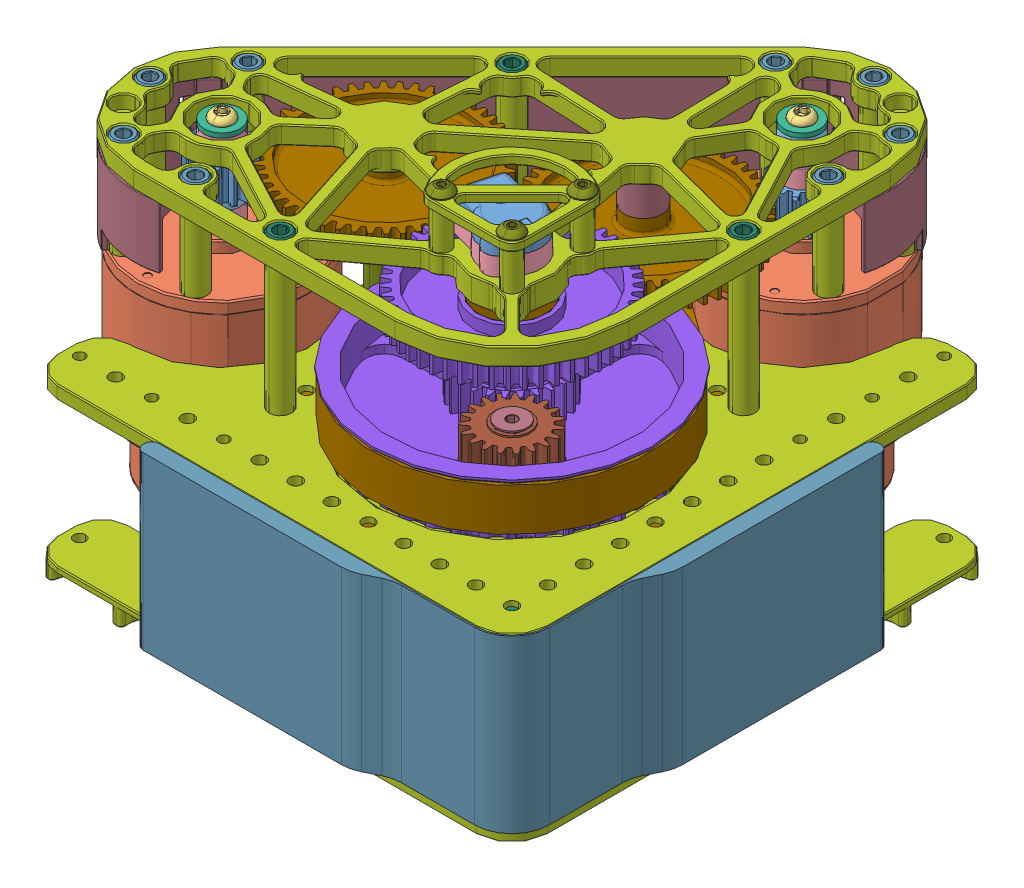
SolidWorks assembly SDS MK4i Swerve Module, Falcons, Independent, configuration Default. Lengths in mm.
Overall size (211.67 191.97 211.67).
99 component instances, 50 part files, 6 mates.
Components (placement in the parent):
- SDS MK4i Swerve Module, Falcons(2)^SDS MK4i Swerve Module, Falcons, Independent-2: SDS MK4i Swerve Module, Falcons(2)^SDS MK4i Swerve Module, Falcons, Independent [Default] at origin size (192.79 191.97 192.79) (virtual)
  - CANcoder Assembly^SDS MK4i Swerve Module, Falcons(2)_SDS MK4i Swerve Module, Falcons, Independent-1: CANcoder Assembly^SDS MK4i Swerve Module, Falcons(2)_SDS MK4i Swerve Module, Falcons, Independent [Default] at (-66.675 132.3975 -66.675) x (-0.260871 0 0.965374) z (0 1 0) size (21.75 26.91 13.52) (virtual)
    - CANcoder Top Housing^CANcoder Assembly_SDS MK4i Swerve Module, Falcons(2)_SDS MK4i Swerve Module, Falcons, Independent-1: CANcoder Top Housing^CANcoder Assembly_SDS MK4i Swerve Module, Falcons(2)_SDS MK4i Swerve Module, Falcons, Independent [Default] at origin size (21.53 26.79 8.94) (virtual)
    - CANcoder PCA^CANcoder Assembly_SDS MK4i Swerve Module, Falcons(2)_SDS MK4i Swerve Module, Falcons, Independent-1: CANcoder PCA^CANcoder Assembly_SDS MK4i Swerve Module, Falcons(2)_SDS MK4i Swerve Module, Falcons, Independent [Default] at (0 0 22.3055) size (15.93 23.27 3.19) (virtual)
    - CANcoder Screw^CANcoder Assembly_SDS MK4i Swerve Module, Falcons(2)_SDS MK4i Swerve Module, Falcons, Independent-1: CANcoder Screw^CANcoder Assembly_SDS MK4i Swerve Module, Falcons(2)_SDS MK4i Swerve Module, Falcons, Independent [Default] at origin size (4.24 4.24 12.65) (virtual)
    - CANcoder Bottom Housing^CANcoder Assembly_SDS MK4i Swerve Module, Falcons(2)_SDS MK4i Swerve Module, Falcons, Independent-1: CANcoder Bottom Housing^CANcoder Assembly_SDS MK4i Swerve Module, Falcons(2)_SDS MK4i Swerve Module, Falcons, Independent [Default] at origin size (21.75 26.91 6.35) (virtual)
  - MK4 Billet Wheel Assembly^SDS MK4i Swerve Module, Falcons(2)_SDS MK4i Swerve Module, Falcons, Independent-1: MK4 Billet Wheel Assembly^SDS MK4i Swerve Module, Falcons(2)_SDS MK4i Swerve Module, Falcons, Independent [Default] at (-66.675 50.7435 -66.675) x (0.707107 0 0.707107) z (0.41117 0.813559 -0.41117) size (42.28 100.13 100.13) (virtual)
    - Wheel, SDS, Nitrile Tread, 4in X 1.5in, Bearing Bore^MK4 Billet Wheel Assembly_SDS MK4i Swerve Module, Falcons(2)_SDS MK4i Swerve Module, Falcons, Independent-1: Wheel, SDS, Nitrile Tread, 4in X 1.5in, Bearing Bore^MK4 Billet Wheel Assembly_SDS MK4i Swerve Module, Falcons(2)_SDS MK4i Swerve Module, Falcons, Independent [Default] at origin size (42.28 88.9 88.9) (virtual)
    - Tread, Blue Nitrile 4in X 1.5in^MK4 Billet Wheel Assembly_SDS MK4i Swerve Module, Falcons(2)_SDS MK4i Swerve Module, Falcons, Independent-1: Tread, Blue Nitrile 4in X 1.5in^MK4 Billet Wheel Assembly_SDS MK4i Swerve Module, Falcons(2)_SDS MK4i Swerve Module, Falcons, Independent [Default] at origin size (38.1 100.13 100.13) (virtual)
    - Screw, 10-32 X .75, Button, 91255A269_91255A269^MK4 Billet Wheel Assembly_SDS MK4i Swerve Module, Falcons(2)_SDS MK4i Swerve Module, Falcons, Independent-1: Screw, 10-32 X .75, Button, 91255A269_91255A269^MK4 Billet Wheel Assembly_SDS MK4i Swerve Module, Falcons(2)_SDS MK4i Swerve Module, Falcons, Independent [Default] at (-4.826 0 20.6375) x (0 -0.847203 -0.531269) z (-1 0 0) size (9.17 9.17 21.62) (virtual)
    - Screw, 10-32 X .75, Button, 91255A269_91255A269^MK4 Billet Wheel Assembly_SDS MK4i Swerve Module, Falcons(2)_SDS MK4i Swerve Module, Falcons, Independent-2: Screw, 10-32 X .75, Button, 91255A269_91255A269^MK4 Billet Wheel Assembly_SDS MK4i Swerve Module, Falcons(2)_SDS MK4i Swerve Module, Falcons, Independent [Default] at (-4.826 -17.8726 10.3187) x (0 -0.99925 -0.038711) z (-1 0 0) size (9.17 9.17 21.62) (virtual)
    - Screw, 10-32 X .75, Button, 91255A269_91255A269^MK4 Billet Wheel Assembly_SDS MK4i Swerve Module, Falcons(2)_SDS MK4i Swerve Module, Falcons, Independent-3: Screw, 10-32 X .75, Button, 91255A269_91255A269^MK4 Billet Wheel Assembly_SDS MK4i Swerve Module, Falcons(2)_SDS MK4i Swerve Module, Falcons, Independent [Default] at (-4.826 -17.8726 -10.3187) x (0 -0.986188 -0.165633) z (-1 0 0) size (9.17 9.17 21.62) (virtual)
    - Screw, 10-32 X .75, Button, 91255A269_91255A269^MK4 Billet Wheel Assembly_SDS MK4i Swerve Module, Falcons(2)_SDS MK4i Swerve Module, Falcons, Independent-4: Screw, 10-32 X .75, Button, 91255A269_91255A269^MK4 Billet Wheel Assembly_SDS MK4i Swerve Module, Falcons(2)_SDS MK4i Swerve Module, Falcons, Independent [Default] at (-4.826 0 -20.6375) x (0 -0.966455 -0.256836) z (-1 0 0) size (9.17 9.17 21.62) (virtual)
    - Screw, 10-32 X .75, Button, 91255A269_91255A269^MK4 Billet Wheel Assembly_SDS MK4i Swerve Module, Falcons(2)_SDS MK4i Swerve Module, Falcons, Independent-5: Screw, 10-32 X .75, Button, 91255A269_91255A269^MK4 Billet Wheel Assembly_SDS MK4i Swerve Module, Falcons(2)_SDS MK4i Swerve Module, Falcons, Independent [Default] at (-4.826 17.8726 -10.3187) x (0 -0.95104 -0.309068) z (-1 0 0) size (9.17 9.17 21.62) (virtual)
    - Screw, 10-32 X .75, Button, 91255A269_91255A269^MK4 Billet Wheel Assembly_SDS MK4i Swerve Module, Falcons(2)_SDS MK4i Swerve Module, Falcons, Independent-6: Screw, 10-32 X .75, Button, 91255A269_91255A269^MK4 Billet Wheel Assembly_SDS MK4i Swerve Module, Falcons(2)_SDS MK4i Swerve Module, Falcons, Independent [Default] at (-4.826 17.8726 10.3187) x (0 -0.947988 -0.318305) z (-1 0 0) size (9.17 9.17 21.62) (virtual)
    - Screw, 10-32 X .5, Button, 97763A232_97763A232^MK4 Billet Wheel Assembly_SDS MK4i Swerve Module, Falcons(2)_SDS MK4i Swerve Module, Falcons, Independent-1: Screw, 10-32 X .5, Button, 97763A232_97763A232^MK4 Billet Wheel Assembly_SDS MK4i Swerve Module, Falcons(2)_SDS MK4i Swerve Module, Falcons, Independent [Default] at (11.1125 -40.6604 7.1695) x (-0.785325 0.107503 0.609678) z (0 -0.984808 0.173648) size (9.17 9.17 15.27) (virtual)
    - Screw, 10-32 X .5, Button, 97763A232_97763A232^MK4 Billet Wheel Assembly_SDS MK4i Swerve Module, Falcons(2)_SDS MK4i Swerve Module, Falcons, Independent-2: Screw, 10-32 X .5, Button, 97763A232_97763A232^MK4 Billet Wheel Assembly_SDS MK4i Swerve Module, Falcons(2)_SDS MK4i Swerve Module, Falcons, Independent [Default] at (-11.1125 -40.6604 7.1695) x (-0.636812 0.133886 0.759306) z (0 -0.984808 0.173648) size (9.17 9.17 15.27) (virtual)
    - Screw, 10-32 X .5, Button, 97763A232_97763A232^MK4 Billet Wheel Assembly_SDS MK4i Swerve Module, Falcons(2)_SDS MK4i Swerve Module, Falcons, Independent-3: Screw, 10-32 X .5, Button, 97763A232_97763A232^MK4 Billet Wheel Assembly_SDS MK4i Swerve Module, Falcons(2)_SDS MK4i Swerve Module, Falcons, Independent [Default] at (-11.1125 -40.6604 -7.1695) x (0.726076 -0.119403 0.677168) z (0 -0.984808 -0.173648) size (9.17 9.17 15.27) (virtual)
    - Screw, 10-32 X .5, Button, 97763A232_97763A232^MK4 Billet Wheel Assembly_SDS MK4i Swerve Module, Falcons(2)_SDS MK4i Swerve Module, Falcons, Independent-4: Screw, 10-32 X .5, Button, 97763A232_97763A232^MK4 Billet Wheel Assembly_SDS MK4i Swerve Module, Falcons(2)_SDS MK4i Swerve Module, Falcons, Independent [Default] at (11.1125 -40.6604 -7.1695) x (0.841108 -0.09392 0.53265) z (0 -0.984808 -0.173648) size (9.17 9.17 15.27) (virtual)
    - Screw, 10-32 X .5, Button, 97763A232_97763A232^MK4 Billet Wheel Assembly_SDS MK4i Swerve Module, Falcons(2)_SDS MK4i Swerve Module, Falcons, Independent-5: Screw, 10-32 X .5, Button, 97763A232_97763A232^MK4 Billet Wheel Assembly_SDS MK4i Swerve Module, Falcons(2)_SDS MK4i Swerve Module, Falcons, Independent [Default] at (-11.1125 20.6438 -35.7562) x (0.804058 -0.514897 -0.297276) z (0 0.5 -0.866025) size (9.17 9.17 15.27) (virtual)
    - Screw, 10-32 X .5, Button, 97763A232_97763A232^MK4 Billet Wheel Assembly_SDS MK4i Swerve Module, Falcons(2)_SDS MK4i Swerve Module, Falcons, Independent-6: Screw, 10-32 X .5, Button, 97763A232_97763A232^MK4 Billet Wheel Assembly_SDS MK4i Swerve Module, Falcons(2)_SDS MK4i Swerve Module, Falcons, Independent [Default] at (11.1125 20.6438 -35.7562) x (0.926716 -0.32542 -0.187881) z (0 0.5 -0.866025) size (9.17 9.17 15.27) (virtual)
    - Screw, 10-32 X .5, Button, 97763A232_97763A232^MK4 Billet Wheel Assembly_SDS MK4i Swerve Module, Falcons(2)_SDS MK4i Swerve Module, Falcons, Independent-7: Screw, 10-32 X .5, Button, 97763A232_97763A232^MK4 Billet Wheel Assembly_SDS MK4i Swerve Module, Falcons(2)_SDS MK4i Swerve Module, Falcons, Independent [Default] at (11.1125 20.6438 35.7562) x (0.200031 0.848523 -0.489895) z (0 0.5 0.866025) size (9.17 9.17 15.27) (virtual)
    - Screw, 10-32 X .5, Button, 97763A232_97763A232^MK4 Billet Wheel Assembly_SDS MK4i Swerve Module, Falcons(2)_SDS MK4i Swerve Module, Falcons, Independent-8: Screw, 10-32 X .5, Button, 97763A232_97763A232^MK4 Billet Wheel Assembly_SDS MK4i Swerve Module, Falcons(2)_SDS MK4i Swerve Module, Falcons, Independent [Default] at (-11.1125 20.6438 35.7562) x (0.515054 0.74232 -0.428579) z (0 0.5 0.866025) size (9.17 9.17 15.27) (virtual)
  - Screw, 10-32 X .25, Button, 91255A261_91255A261^SDS MK4i Swerve Module, Falcons(2)_SDS MK4i Swerve Module, Falcons, Independent-1: Screw, 10-32 X .25, Button, 91255A261_91255A261^SDS MK4i Swerve Module, Falcons(2)_SDS MK4i Swerve Module, Falcons, Independent [Default] at (-42.2285 89.5096 -114.6539) x (1 0 0) z (0 -1 0) size (9.17 9.17 8.92) (virtual)
  - Screw, 10-32 X .25, Button, 91255A261_91255A261^SDS MK4i Swerve Module, Falcons(2)_SDS MK4i Swerve Module, Falcons, Independent-2: Screw, 10-32 X .25, Button, 91255A261_91255A261^SDS MK4i Swerve Module, Falcons(2)_SDS MK4i Swerve Module, Falcons, Independent [Default] at (-104.7513 89.5096 -104.7513) x (0.982082 0 -0.188455) z (0 -1 0) size (9.17 9.17 8.92) (virtual)
  - Screw, 10-32 X .25, Button, 91255A261_91255A261^SDS MK4i Swerve Module, Falcons(2)_SDS MK4i Swerve Module, Falcons, Independent-3: Screw, 10-32 X .25, Button, 91255A261_91255A261^SDS MK4i Swerve Module, Falcons(2)_SDS MK4i Swerve Module, Falcons, Independent [Default] at (-114.6539 89.5096 -42.2285) x (0.918365 0 -0.395734) z (0 -1 0) size (9.17 9.17 8.92) (virtual)
  - Screw, 10-32 X .25, Button, 91255A261_91255A261^SDS MK4i Swerve Module, Falcons(2)_SDS MK4i Swerve Module, Falcons, Independent-4: Screw, 10-32 X .25, Button, 91255A261_91255A261^SDS MK4i Swerve Module, Falcons(2)_SDS MK4i Swerve Module, Falcons, Independent [Default] at (-63.5129 89.5096 -12.9199) x (0.8 0 -0.6) z (0 -1 0) size (9.17 9.17 8.92) (virtual)
  - Screw, 10-32 X .25, Button, 91255A261_91255A261^SDS MK4i Swerve Module, Falcons(2)_SDS MK4i Swerve Module, Falcons, Independent-5: Screw, 10-32 X .25, Button, 91255A261_91255A261^SDS MK4i Swerve Module, Falcons(2)_SDS MK4i Swerve Module, Falcons, Independent [Default] at (-12.9199 89.5096 -63.5129) x (0.63358 0 -0.773678) z (0 -1 0) size (9.17 9.17 8.92) (virtual)
  - Screw, Shoulder, .375 X 2.5, 5_16-18, 91259A634_91259A634^SDS MK4i Swerve Module, Falcons(2)_SDS MK4i Swerve Module, Falcons, Independent-1: Screw, Shoulder, .375 X 2.5, 5_16-18, 91259A634_91259A634^SDS MK4i Swerve Module, Falcons(2)_SDS MK4i Swerve Module, Falcons, Independent [Default] at (-93.8403 50.7435 -93.8403) x (-0.019195 -0.999631 0.019195) z (0.706846 -0.027146 -0.706846) size (14.29 82.55 14.29) (virtual)
  - Screw, .25-20 X 1 Socket, 91251A542_91251A542^SDS MK4i Swerve Module, Falcons(2)_SDS MK4i Swerve Module, Falcons, Independent-1: Screw, .25-20 X 1 Socket, 91251A542_91251A542^SDS MK4i Swerve Module, Falcons(2)_SDS MK4i Swerve Module, Falcons, Independent [Default] at (-102.596 101.6 -73.8592) x (0.964329 0 0.264706) z (0 1 0) size (9.53 9.53 31.75) (virtual)
  - Screw, .25-20 X 1 Socket, 91251A542_91251A542^SDS MK4i Swerve Module, Falcons(2)_SDS MK4i Swerve Module, Falcons, Independent-2: Screw, .25-20 X 1 Socket, 91251A542_91251A542^SDS MK4i Swerve Module, Falcons(2)_SDS MK4i Swerve Module, Falcons, Independent [Default] at (-73.8592 101.6 -102.596) x (0.982082 0 -0.188455) z (0 1 0) size (9.53 9.53 31.75) (virtual)
  - Screw, .25-20 X .625, 91251A539_91251A539^SDS MK4i Swerve Module, Falcons(2)_SDS MK4i Swerve Module, Falcons, Independent-1: Screw, .25-20 X .625, 91251A539_91251A539^SDS MK4i Swerve Module, Falcons(2)_SDS MK4i Swerve Module, Falcons, Independent [Default] at (-59.4908 83.2802 -30.754) x (1 0 0) z (0 -1 0) size (9.53 9.53 22.23) (virtual)
  - Screw, .25-20 X .625, 91251A539_91251A539^SDS MK4i Swerve Module, Falcons(2)_SDS MK4i Swerve Module, Falcons, Independent-2: Screw, .25-20 X .625, 91251A539_91251A539^SDS MK4i Swerve Module, Falcons(2)_SDS MK4i Swerve Module, Falcons, Independent [Default] at (-30.754 83.2802 -59.4908) x (0.982082 0 -0.188455) z (0 -1 0) size (9.53 9.53 22.23) (virtual)
  - Screw, .25-20 X .625, 91251A539_91251A539^SDS MK4i Swerve Module, Falcons(2)_SDS MK4i Swerve Module, Falcons, Independent-3: Screw, .25-20 X .625, 91251A539_91251A539^SDS MK4i Swerve Module, Falcons(2)_SDS MK4i Swerve Module, Falcons, Independent [Default] at (-66.675 126.2062 -66.675) x (0 0 1) z (0 1 0) size (9.53 9.53 22.23) (virtual)
  - Screw, 12-24 X .625, Flat, 91253A282_91253A282^SDS MK4i Swerve Module, Falcons(2)_SDS MK4i Swerve Module, Falcons, Independent-1: Screw, 12-24 X .625, Flat, 91253A282_91253A282^SDS MK4i Swerve Module, Falcons(2)_SDS MK4i Swerve Module, Falcons, Independent [Default] at (-46.8646 122.8979 -46.8646) x (-0.837169 0 -0.546944) z (0 1 0) size (10.72 10.72 15.88) (virtual)
  - Screw, 10-32 X 1.375, 90044A202_90044A202^SDS MK4i Swerve Module, Falcons(2)_SDS MK4i Swerve Module, Falcons, Independent-1: Screw, 10-32 X 1.375, 90044A202_90044A202^SDS MK4i Swerve Module, Falcons(2)_SDS MK4i Swerve Module, Falcons, Independent [Default] at (-34.518 138.8491 -146.05) x (-0.434408 0 0.900716) z (0 1 0) size (7.94 7.94 39.75) (virtual)
  - Screw, 10-32 X 1.375, 90044A202_90044A202^SDS MK4i Swerve Module, Falcons(2)_SDS MK4i Swerve Module, Falcons, Independent-2: Screw, 10-32 X 1.375, 90044A202_90044A202^SDS MK4i Swerve Module, Falcons(2)_SDS MK4i Swerve Module, Falcons, Independent [Default] at (-34.518 138.8491 -171.45) x (-0.25688 0 0.966443) z (0 1 0) size (7.94 7.94 39.75) (virtual)
  - Screw, 10-32 X 1.375, 90044A202_90044A202^SDS MK4i Swerve Module, Falcons(2)_SDS MK4i Swerve Module, Falcons, Independent-3: Screw, 10-32 X 1.375, 90044A202_90044A202^SDS MK4i Swerve Module, Falcons(2)_SDS MK4i Swerve Module, Falcons, Independent [Default] at (-56.515 138.8491 -184.15) x (-0.042501 0 0.999096) z (0 1 0) size (7.94 7.94 39.75) (virtual)
  - Screw, 10-32 X 1.375, 90044A202_90044A202^SDS MK4i Swerve Module, Falcons(2)_SDS MK4i Swerve Module, Falcons, Independent-4: Screw, 10-32 X 1.375, 90044A202_90044A202^SDS MK4i Swerve Module, Falcons(2)_SDS MK4i Swerve Module, Falcons, Independent [Default] at (-78.512 138.8491 -171.45) x (0.192903 0 0.981218) z (0 1 0) size (7.94 7.94 39.75) (virtual)
  - Screw, 10-32 X 1.375, 90044A202_90044A202^SDS MK4i Swerve Module, Falcons(2)_SDS MK4i Swerve Module, Falcons, Independent-5: Screw, 10-32 X 1.375, 90044A202_90044A202^SDS MK4i Swerve Module, Falcons(2)_SDS MK4i Swerve Module, Falcons, Independent [Default] at (-171.45 138.8491 -78.512) x (0.421632 0 0.906767) z (0 1 0) size (7.94 7.94 39.75) (virtual)
  - Screw, 10-32 X 1.375, 90044A202_90044A202^SDS MK4i Swerve Module, Falcons(2)_SDS MK4i Swerve Module, Falcons, Independent-6: Screw, 10-32 X 1.375, 90044A202_90044A202^SDS MK4i Swerve Module, Falcons(2)_SDS MK4i Swerve Module, Falcons, Independent [Default] at (-184.15 138.8491 -56.515) x (0.614515 0 0.788905) z (0 1 0) size (7.94 7.94 39.75) (virtual)
  - Screw, 10-32 X 1.375, 90044A202_90044A202^SDS MK4i Swerve Module, Falcons(2)_SDS MK4i Swerve Module, Falcons, Independent-7: Screw, 10-32 X 1.375, 90044A202_90044A202^SDS MK4i Swerve Module, Falcons(2)_SDS MK4i Swerve Module, Falcons, Independent [Default] at (-171.45 138.8491 -34.518) x (0.754605 0 0.656179) z (0 1 0) size (7.94 7.94 39.75) (virtual)
  - Screw, 10-32 X 1.375, 90044A202_90044A202^SDS MK4i Swerve Module, Falcons(2)_SDS MK4i Swerve Module, Falcons, Independent-8: Screw, 10-32 X 1.375, 90044A202_90044A202^SDS MK4i Swerve Module, Falcons(2)_SDS MK4i Swerve Module, Falcons, Independent [Default] at (-146.05 138.8491 -34.518) x (0.201272 0 -0.979535) z (0 1 0) size (7.94 7.94 39.75) (virtual)
  - Screw, 10-32 X 2.25, 91251A354_91251A354^SDS MK4i Swerve Module, Falcons(2)_SDS MK4i Swerve Module, Falcons, Independent-1: Screw, 10-32 X 2.25, 91251A354_91251A354^SDS MK4i Swerve Module, Falcons(2)_SDS MK4i Swerve Module, Falcons, Independent [Default] at (-124.5154 92.0115 -124.5154) x (-0.750514 0 0.660855) z (0 -1 0) size (7.92 7.92 61.98) (virtual)
  - Screw, 10-32 X 2.25, 91251A354_91251A354^SDS MK4i Swerve Module, Falcons(2)_SDS MK4i Swerve Module, Falcons, Independent-2: Screw, 10-32 X 2.25, 91251A354_91251A354^SDS MK4i Swerve Module, Falcons(2)_SDS MK4i Swerve Module, Falcons, Independent [Default] at (-32.639 92.0115 -114.3) x (-0.612525 0 0.790452) z (0 -1 0) size (7.92 7.92 61.98) (virtual)
  - Screw, 10-32 X 2.25, 91251A354_91251A354^SDS MK4i Swerve Module, Falcons(2)_SDS MK4i Swerve Module, Falcons, Independent-3: Screw, 10-32 X 2.25, 91251A354_91251A354^SDS MK4i Swerve Module, Falcons(2)_SDS MK4i Swerve Module, Falcons, Independent [Default] at (-114.3 92.0115 -32.639) x (-0.427723 0 0.90391) z (0 -1 0) size (7.92 7.92 61.98) (virtual)
  - Screw, 10-32 X 2.25, 91251A354_91251A354^SDS MK4i Swerve Module, Falcons(2)_SDS MK4i Swerve Module, Falcons, Independent-4: Screw, 10-32 X 2.25, 91251A354_91251A354^SDS MK4i Swerve Module, Falcons(2)_SDS MK4i Swerve Module, Falcons, Independent [Default] at (-12.7 98.4885 -12.7) x (0.90391 0 -0.427723) z (0 1 0) size (7.92 7.92 61.98) (virtual)
  - Screw, 8-32 X .875, Button, 91255A166_91255A166^SDS MK4i Swerve Module, Falcons(2)_SDS MK4i Swerve Module, Falcons, Independent-1: Screw, 8-32 X .875, Button, 91255A166_91255A166^SDS MK4i Swerve Module, Falcons(2)_SDS MK4i Swerve Module, Falcons, Independent [Default] at (-80.9791 172.8661 -56.1146) x (1 0 0) z (0 1 0) size (7.92 7.92 24.45) (virtual)
  - Screw, 8-32 X .875, Button, 91255A166_91255A166^SDS MK4i Swerve Module, Falcons(2)_SDS MK4i Swerve Module, Falcons, Independent-2: Screw, 8-32 X .875, Button, 91255A166_91255A166^SDS MK4i Swerve Module, Falcons(2)_SDS MK4i Swerve Module, Falcons, Independent [Default] at (-56.1231 172.8661 -56.1146) x (0.982082 0 -0.188455) z (0 1 0) size (7.92 7.92 24.45) (virtual)
  - Screw, 8-32 X .875, Button, 91255A166_91255A166^SDS MK4i Swerve Module, Falcons(2)_SDS MK4i Swerve Module, Falcons, Independent-3: Screw, 8-32 X .875, Button, 91255A166_91255A166^SDS MK4i Swerve Module, Falcons(2)_SDS MK4i Swerve Module, Falcons, Independent [Default] at (-56.1231 172.8661 -80.9854) x (0.918365 0 -0.395734) z (0 1 0) size (7.92 7.92 24.45) (virtual)
  - Shim, 8mm ID X 14mm OD X .5mm Thick, 98055A115_98055A115^SDS MK4i Swerve Module, Falcons(2)_SDS MK4i Swerve Module, Falcons, Independent-1: Shim, 8mm ID X 14mm OD X .5mm Thick, 98055A115_98055A115^SDS MK4i Swerve Module, Falcons(2)_SDS MK4i Swerve Module, Falcons, Independent [Default] at (-46.8646 73.9775 -46.8646) x (0.942304 0 -0.334759) z (0.334759 0 0.942304) size (14 1 14) (virtual)
  - Bearing, 6802^SDS MK4i Swerve Module, Falcons(2)_SDS MK4i Swerve Module, Falcons, Independent-1: Bearing, 6802^SDS MK4i Swerve Module, Falcons(2)_SDS MK4i Swerve Module, Falcons, Independent [Default] at (-66.675 138.5216 -66.675) x (0.972423 0 0.233226) z (-0.233226 0 0.972423) size (24 5 24) (virtual)
  - Bearing, 6802^SDS MK4i Swerve Module, Falcons(2)_SDS MK4i Swerve Module, Falcons, Independent-2: Bearing, 6802^SDS MK4i Swerve Module, Falcons(2)_SDS MK4i Swerve Module, Falcons, Independent [Default] at (-66.675 147.8675 -66.675) x (0.877163 0 0.480193) z (-0.480193 0 0.877163) size (24 5 24) (virtual)
  - Bearing, 6802^SDS MK4i Swerve Module, Falcons(2)_SDS MK4i Swerve Module, Falcons, Independent-3: Bearing, 6802^SDS MK4i Swerve Module, Falcons(2)_SDS MK4i Swerve Module, Falcons, Independent [Default] at (-66.675 118.1216 -66.675) x (0.639486 0 0.768802) z (-0.768802 0 0.639486) size (24 5 24) (virtual)
  - Bearing, R6ZZ^SDS MK4i Swerve Module, Falcons(2)_SDS MK4i Swerve Module, Falcons, Independent-1: Bearing, R6ZZ^SDS MK4i Swerve Module, Falcons(2)_SDS MK4i Swerve Module, Falcons, Independent [Default] at (-79.2721 50.7435 -79.2721) x (-0.694824 0.18558 0.694824) z (0.131225 0.982629 -0.131225) size (22.23 7.14 22.23) (virtual)
  - Bearing, R8ZZ^SDS MK4i Swerve Module, Falcons(2)_SDS MK4i Swerve Module, Falcons, Independent-1: Bearing, R8ZZ^SDS MK4i Swerve Module, Falcons(2)_SDS MK4i Swerve Module, Falcons, Independent [Default] at (-57.5286 50.7435 -57.5286) x (-0.158587 -0.974526 0.158587) z (-0.689094 0.224275 0.689094) size (28.57 7.94 28.57) (virtual)
  - Bearing, 688^SDS MK4i Swerve Module, Falcons(2)_SDS MK4i Swerve Module, Falcons, Independent-1: Bearing, 688^SDS MK4i Swerve Module, Falcons(2)_SDS MK4i Swerve Module, Falcons, Independent [Default] at (-46.8646 71.4775 -46.8646) x (0 -1 0) z (-0.336154 0 0.941807) size (5 16 16) (virtual)
  - Bearing, .375 ThunderHex, Flanged, 217-5829^SDS MK4i Swerve Module, Falcons(2)_SDS MK4i Swerve Module, Falcons, Independent-1: Bearing, .375 ThunderHex, Flanged, 217-5829^SDS MK4i Swerve Module, Falcons(2)_SDS MK4i Swerve Module, Falcons, Independent [Default] at (-46.8646 102.3938 -46.8646) x (0.903016 0 0.429606) z (-0.429606 0 0.903016) size (24.51 7.14 24.51) (virtual)
  - Bevel Gear, 1545^SDS MK4i Swerve Module, Falcons(2)_SDS MK4i Swerve Module, Falcons, Independent-1: Bevel Gear, 1545^SDS MK4i Swerve Module, Falcons(2)_SDS MK4i Swerve Module, Falcons, Independent [Default] at (-46.8646 84.4935 -46.8646) x (-0.830686 0 -0.556741) z (-0.556741 0 0.830686) size (28.28 15.37 25.62) (virtual)
  - Bearing, 688^SDS MK4i Swerve Module, Falcons(2)_SDS MK4i Swerve Module, Falcons, Independent-2: Bearing, 688^SDS MK4i Swerve Module, Falcons(2)_SDS MK4i Swerve Module, Falcons, Independent [Default] at (-128.0498 97.5125 -83.2602) x (0 -1 0) z (-0.444562 0 0.895748) size (5 16 16) (virtual)
  - Bearing, R188ZZ, 217-3489^SDS MK4i Swerve Module, Falcons(2)_SDS MK4i Swerve Module, Falcons, Independent-1: Bearing, R188ZZ, 217-3489^SDS MK4i Swerve Module, Falcons(2)_SDS MK4i Swerve Module, Falcons, Independent [Default] at (-77.6314 97.6313 -123.9376) x (-0.188457 0 -0.982081) z (0.982081 0 -0.188457) size (12.7 4.76 12.7) (virtual)
  - Bearing, 688^SDS MK4i Swerve Module, Falcons(2)_SDS MK4i Swerve Module, Falcons, Independent-3: Bearing, 688^SDS MK4i Swerve Module, Falcons(2)_SDS MK4i Swerve Module, Falcons, Independent [Default] at (-77.6314 150.1375 -123.9376) x (0 -1 0) z (-0.336154 0 0.941807) size (5 16 16) (virtual)
  - Bearing, 688^SDS MK4i Swerve Module, Falcons(2)_SDS MK4i Swerve Module, Falcons, Independent-4: Bearing, 688^SDS MK4i Swerve Module, Falcons(2)_SDS MK4i Swerve Module, Falcons, Independent [Default] at (-128.0498 148.8167 -83.2602) x (0 -1 0) z (-0.336154 0 0.941807) size (5 16 16) (virtual)
  - Bearing, A035XPO_SA035XPO^SDS MK4i Swerve Module, Falcons(2)_SDS MK4i Swerve Module, Falcons, Independent-1: Bearing, A035XPO_SA035XPO^SDS MK4i Swerve Module, Falcons(2)_SDS MK4i Swerve Module, Falcons, Independent [Default] at (-66.675 95.25 -66.675) x (0.978935 0 0.20417) z (-0.20417 0 0.978935) size (101.6 6.35 101.6) (virtual)
  - Double Gear, 20DP, 25T, 50T^SDS MK4i Swerve Module, Falcons(2)_SDS MK4i Swerve Module, Falcons, Independent-1: Double Gear, 20DP, 25T, 50T^SDS MK4i Swerve Module, Falcons(2)_SDS MK4i Swerve Module, Falcons, Independent [Default] at (-66.675 110.1225 -66.675) x (-0.730582 0 -0.682825) z (0 1 0) size (65.97 66.04 34.49) (virtual)
  - Gear, 50T, 20DP, .375Hex^SDS MK4i Swerve Module, Falcons(2)_SDS MK4i Swerve Module, Falcons, Independent-1: Gear, 50T, 20DP, .375Hex^SDS MK4i Swerve Module, Falcons(2)_SDS MK4i Swerve Module, Falcons, Independent [Default] at (-128.0498 139.8651 -83.2602) x (0.985885 0 -0.167422) z (0 1 0) size (65.97 66.04 12.65) (virtual)
  - Gear, 50T, 20DP, .375Hex^SDS MK4i Swerve Module, Falcons(2)_SDS MK4i Swerve Module, Falcons, Independent-2: Gear, 50T, 20DP, .375Hex^SDS MK4i Swerve Module, Falcons(2)_SDS MK4i Swerve Module, Falcons, Independent [Default] at (-77.6314 128.4859 -123.9376) x (-0.963721 0 0.266911) z (0 1 0) size (65.97 66.04 12.65) (virtual)
  - Bevel Gear, 4515^SDS MK4i Swerve Module, Falcons(2)_SDS MK4i Swerve Module, Falcons, Independent-1: Bevel Gear, 4515^SDS MK4i Swerve Module, Falcons(2)_SDS MK4i Swerve Module, Falcons, Independent [Default] at (-54.7746 50.7435 -54.7746) x (0.575273 -0.581482 -0.575273) z (-0.41117 -0.813559 0.41117) size (68.38 7.77 68.42) (virtual)
  - Gear, 19T, 20DP, .375Hex^SDS MK4i Swerve Module, Falcons(2)_SDS MK4i Swerve Module, Falcons, Independent-1: Gear, 19T, 20DP, .375Hex^SDS MK4i Swerve Module, Falcons(2)_SDS MK4i Swerve Module, Falcons, Independent [Default] at (-46.8646 115.8367 -46.8646) x (0.115868 0 -0.993265) z (0.993265 0 0.115868) size (26.55 12.6 26.64) (virtual)
  - MK4i Steering Shaft Tall^SDS MK4i Swerve Module, Falcons(2)_SDS MK4i Swerve Module, Falcons, Independent-1: MK4i Steering Shaft Tall^SDS MK4i Swerve Module, Falcons(2)_SDS MK4i Swerve Module, Falcons, Independent [Default] at (-77.6314 152.5105 -123.9376) x (0.998641 0 -0.05212) z (0.05212 0 0.998641) size (17.78 57.04 17.78) (virtual)
  - MK4i Steering Shaft Spacer^SDS MK4i Swerve Module, Falcons(2)_SDS MK4i Swerve Module, Falcons, Independent-1: MK4i Steering Shaft Spacer^SDS MK4i Swerve Module, Falcons(2)_SDS MK4i Swerve Module, Falcons, Independent [Default] at (-77.6314 134.8105 -123.9376) x (-0.728275 0 -0.685285) z (0.685285 0 -0.728275) size (13.36 12.7 13.36) (virtual)
  - MK4 Intermediate Shaft^SDS MK4i Swerve Module, Falcons(2)_SDS MK4i Swerve Module, Falcons, Independent-1: MK4 Intermediate Shaft^SDS MK4i Swerve Module, Falcons(2)_SDS MK4i Swerve Module, Falcons, Independent [Default] at (-46.8646 68.3577 -46.8646) x (0.999953 0 0.009669) z (-0.009669 0 0.999953) size (11.68 51.44 11.68) (virtual)
  - MK3 Center Column^SDS MK4i Swerve Module, Falcons(2)_SDS MK4i Swerve Module, Falcons, Independent-1: MK3 Center Column^SDS MK4i Swerve Module, Falcons(2)_SDS MK4i Swerve Module, Falcons, Independent [Default] at (-66.675 113.0816 -66.675) x (-0.707107 0 0.707107) z (-0.707107 0 -0.707107) size (17.27 40.32 17.27) (virtual)
  - MK4i Shaft, Drive Idler^SDS MK4i Swerve Module, Falcons(2)_SDS MK4i Swerve Module, Falcons, Independent-1: MK4i Shaft, Drive Idler^SDS MK4i Swerve Module, Falcons(2)_SDS MK4i Swerve Module, Falcons, Independent [Default] at (-128.0498 100.0125 -83.2602) size (13.36 56.18 13.36) (virtual)
  - Screw, 3-48 X .1875, Pan Phillips, 90272A091_90272A091^SDS MK4i Swerve Module, Falcons(2)_SDS MK4i Swerve Module, Falcons, Independent-1: Screw, 3-48 X .1875, Pan Phillips, 90272A091_90272A091^SDS MK4i Swerve Module, Falcons(2)_SDS MK4i Swerve Module, Falcons, Independent [Default] at (-68.5859 150.495 -73.8677) x (1 0 0) z (0 1 0) size (4.9 4.9 6.49) (virtual)
  - Screw, 3-48 X .1875, Pan Phillips, 90272A091_90272A091^SDS MK4i Swerve Module, Falcons(2)_SDS MK4i Swerve Module, Falcons, Independent-2: Screw, 3-48 X .1875, Pan Phillips, 90272A091_90272A091^SDS MK4i Swerve Module, Falcons(2)_SDS MK4i Swerve Module, Falcons, Independent [Default] at (-64.7641 150.495 -59.4823) x (0.911631 0 -0.411009) z (0 1 0) size (4.9 4.9 6.49) (virtual)
  - magnet^SDS MK4i Swerve Module, Falcons(2)_SDS MK4i Swerve Module, Falcons, Independent-1: magnet^SDS MK4i Swerve Module, Falcons(2)_SDS MK4i Swerve Module, Falcons, Independent [Default] at (-66.675 140.7033 -66.675) x (-0.536649 0 -0.843806) z (0.843806 0 -0.536649) size (6.35 12.7 6.35) (virtual)
  - Gear, 20DP 14T, Falcon Spline, am-4147^SDS MK4i Swerve Module, Falcons(2)_SDS MK4i Swerve Module, Falcons, Independent-1: Gear, 20DP 14T, Falcon Spline, am-4147^SDS MK4i Swerve Module, Falcons(2)_SDS MK4i Swerve Module, Falcons, Independent [Default] at (-56.515 123.7 -158.75) x (0 1 0) z (-0.155924 0 -0.987769) size (12.71 19.97 20.32) (virtual)
  - Gear, 20DP 14T, Falcon Spline, am-4147^SDS MK4i Swerve Module, Falcons(2)_SDS MK4i Swerve Module, Falcons, Independent-2: Gear, 20DP 14T, Falcon Spline, am-4147^SDS MK4i Swerve Module, Falcons(2)_SDS MK4i Swerve Module, Falcons, Independent [Default] at (-158.75 133.225 -56.515) x (0 1 0) z (-0.622557 0 -0.782574) size (12.71 19.97 20.32) (virtual)
  - Motor, Falcon500^SDS MK4i Swerve Module, Falcons(2)_SDS MK4i Swerve Module, Falcons, Independent-1: Motor, Falcon500^SDS MK4i Swerve Module, Falcons(2)_SDS MK4i Swerve Module, Falcons, Independent [Default] at (-158.75 82.1244 -56.515) x (0 0 1) z (0 1 0) size (61.56 60.51 116.08) (virtual)
  - Motor, Falcon500^SDS MK4i Swerve Module, Falcons(2)_SDS MK4i Swerve Module, Falcons, Independent-2: Motor, Falcon500^SDS MK4i Swerve Module, Falcons(2)_SDS MK4i Swerve Module, Falcons, Independent [Default] at (-56.515 82.1244 -158.75) x (-1 0 0) z (0 1 0) size (61.56 60.51 116.08) (virtual)
  - Screw, Falcon 500 Pinion_90939A124^SDS MK4i Swerve Module, Falcons(2)_SDS MK4i Swerve Module, Falcons, Independent-1: Screw, Falcon 500 Pinion_90939A124^SDS MK4i Swerve Module, Falcons(2)_SDS MK4i Swerve Module, Falcons, Independent [Default] at (-56.515 153.8625 -158.75) x (1 0 0) z (0 1 0) size (7.93 7.93 14.91) (virtual)
  - Screw, Falcon 500 Pinion_90939A124^SDS MK4i Swerve Module, Falcons(2)_SDS MK4i Swerve Module, Falcons, Independent-2: Screw, Falcon 500 Pinion_90939A124^SDS MK4i Swerve Module, Falcons(2)_SDS MK4i Swerve Module, Falcons, Independent [Default] at (-158.75 153.8625 -56.515) x (0.982082 0 -0.188455) z (0 1 0) size (7.93 7.93 14.91) (virtual)
  - Falcon Spacer .25^SDS MK4i Swerve Module, Falcons(2)_SDS MK4i Swerve Module, Falcons, Independent-1: Falcon Spacer .25^SDS MK4i Swerve Module, Falcons(2)_SDS MK4i Swerve Module, Falcons, Independent [Default] at (-56.515 136.4 -158.75) size (12.7 6.35 12.7) (virtual)
  - Falcon Spacer .25^SDS MK4i Swerve Module, Falcons(2)_SDS MK4i Swerve Module, Falcons, Independent-2: Falcon Spacer .25^SDS MK4i Swerve Module, Falcons(2)_SDS MK4i Swerve Module, Falcons, Independent [Default] at (-56.515 142.75 -158.75) x (0.982082 0 -0.188455) z (0.188455 0 0.982082) size (12.7 6.35 12.7) (virtual)
  - Falcon Spacer .25^SDS MK4i Swerve Module, Falcons(2)_SDS MK4i Swerve Module, Falcons, Independent-3: Falcon Spacer .25^SDS MK4i Swerve Module, Falcons(2)_SDS MK4i Swerve Module, Falcons, Independent [Default] at (-158.75 123.7 -56.515) x (0.995401 0 0.095792) z (-0.095792 0 0.995401) size (12.7 6.35 12.7) (virtual)
  - Falcon Spacer .25^SDS MK4i Swerve Module, Falcons(2)_SDS MK4i Swerve Module, Falcons, Independent-4: Falcon Spacer .25^SDS MK4i Swerve Module, Falcons(2)_SDS MK4i Swerve Module, Falcons, Independent [Default] at (-158.75 145.925 -56.515) x (0.92897 0 -0.370156) z (0.370156 0 0.92897) size (12.7 6.35 12.7) (virtual)
  - Falcon Spacer .125^SDS MK4i Swerve Module, Falcons(2)_SDS MK4i Swerve Module, Falcons, Independent-1: Falcon Spacer .125^SDS MK4i Swerve Module, Falcons(2)_SDS MK4i Swerve Module, Falcons, Independent [Default] at (-56.515 149.1 -158.75) x (0.944247 0 -0.329237) z (0.329237 0 0.944247) size (12.7 3.17 12.7) (virtual)
  - Falcon Spacer .125^SDS MK4i Swerve Module, Falcons(2)_SDS MK4i Swerve Module, Falcons, Independent-2: Falcon Spacer .125^SDS MK4i Swerve Module, Falcons(2)_SDS MK4i Swerve Module, Falcons, Independent [Default] at (-158.75 130.05 -56.515) x (0.865282 0 -0.501286) z (0.501286 0 0.865282) size (12.7 3.17 12.7) (virtual)
  - Falcon Spacer .0625^SDS MK4i Swerve Module, Falcons(2)_SDS MK4i Swerve Module, Falcons, Independent-1: Falcon Spacer .0625^SDS MK4i Swerve Module, Falcons(2)_SDS MK4i Swerve Module, Falcons, Independent [Default] at (-158.75 152.275 -56.515) size (12.7 1.59 12.7) (virtual)
  - Falcon Spacer .0625^SDS MK4i Swerve Module, Falcons(2)_SDS MK4i Swerve Module, Falcons, Independent-2: Falcon Spacer .0625^SDS MK4i Swerve Module, Falcons(2)_SDS MK4i Swerve Module, Falcons, Independent [Default] at (-56.515 152.275 -158.75) x (0.982082 0 -0.188455) z (0.188455 0 0.982082) size (12.7 1.59 12.7) (virtual)
  - MK4i Master Part_Default Falcon 500 Config^SDS MK4i Swerve Module, Falcons(2)_SDS MK4i Swerve Module, Falcons, Independent-1: MK4i Master Part_Default Falcon 500 Config^SDS MK4i Swerve Module, Falcons(2)_SDS MK4i Swerve Module, Falcons, Independent [Default] at origin size (189.87 134.14 189.87) (virtual)
  - MK3 Base Pulley Tall^SDS MK4i Swerve Module, Falcons(2)_SDS MK4i Swerve Module, Falcons, Independent-1: MK3 Base Pulley Tall^SDS MK4i Swerve Module, Falcons(2)_SDS MK4i Swerve Module, Falcons, Independent [Default] at (-66.675 98.425 -66.675) x (-0.707107 0 0.707107) z (-0.707107 0 -0.707107) size (98.42 27.08 98.42) (virtual)
  - Belt, 320-5M-15^SDS MK4i Swerve Module, Falcons(2)_SDS MK4i Swerve Module, Falcons, Independent-1: Belt, 320-5M-15^SDS MK4i Swerve Module, Falcons(2)_SDS MK4i Swerve Module, Falcons, Independent [Default] at (-66.675 109.752 -66.675) x (0.982183 0 -0.187927) z (0.187927 0 0.982183) size (97.78 15 116.29) (virtual)
  - Wheel Mount A^SDS MK4i Swerve Module, Falcons(2)_SDS MK4i Swerve Module, Falcons, Independent-1: Wheel Mount A^SDS MK4i Swerve Module, Falcons(2)_SDS MK4i Swerve Module, Falcons, Independent [Default] at (-88.2276 50.7435 -88.2276) x (-0.707107 0 -0.707107) z (0.707107 0 -0.707107) size (17.09 49.74 57.15) (virtual)
  - Wheel Mount B Gen2^SDS MK4i Swerve Module, Falcons(2)_SDS MK4i Swerve Module, Falcons, Independent-1: Wheel Mount B Gen2^SDS MK4i Swerve Module, Falcons(2)_SDS MK4i Swerve Module, Falcons, Independent [Default] at (-45.1224 50.7435 -45.1224) x (-0.707107 0 -0.707107) z (0.707107 0 -0.707107) size (15.88 49.27 57.15) (virtual)
  - MK4 Wheel Spacer^SDS MK4i Swerve Module, Falcons(2)_SDS MK4i Swerve Module, Falcons, Independent-1: MK4 Wheel Spacer^SDS MK4i Swerve Module, Falcons(2)_SDS MK4i Swerve Module, Falcons, Independent [Default] at (-76.7015 50.7435 -76.7015) x (-0.707107 0 -0.707107) z (0.522819 -0.67329 -0.522819) size (36.72 15.11 15.11) (virtual)
- swervecover-1: swervecover [Default] at (-107.6325 133.3754 -107.6325) x (-0.707107 0 0.707107) z (-0.707107 0 -0.707107) size (206.81 50.4 62.67)
- bumper legalizer-1: bumper legalizer [Default] at (-12.7 44.45 -12.7) size (124.66 60.33 124.66)
Mates (geometry in assembly coordinates):
- Concentric9: concentric aligned: cylinder of SDS MK4i Swerve Module, Falcons(2)^SDS MK4i Swerve Module, Falcons, Independent-2/MK4i Master Part_Default Falcon 500 Config^SDS MK4i Swerve Module, Falcons(2)_SDS MK4i Swerve Module, Falcons, Independent-1 through (-56.515 153.9875 -158.75) axis (0 -1 0) radius 31.115; cylinder of swervecover-1 through (-56.515 147.6375 -158.75) axis (0 -1 0) radius 29.3687
- Concentric10: concentric aligned: cylinder of SDS MK4i Swerve Module, Falcons(2)^SDS MK4i Swerve Module, Falcons, Independent-2/MK4i Master Part_Default Falcon 500 Config^SDS MK4i Swerve Module, Falcons(2)_SDS MK4i Swerve Module, Falcons, Independent-1 through (-158.75 153.9875 -56.515) axis (0 -1 0) radius 31.115; cylinder of swervecover-1 through (-158.75 147.6375 -56.515) axis (0 -1 0) radius 29.3687
- Coincident3: coincident anti-aligned: plane of SDS MK4i Swerve Module, Falcons(2)^SDS MK4i Swerve Module, Falcons, Independent-2/MK4i Master Part_Default Falcon 500 Config^SDS MK4i Swerve Module, Falcons(2)_SDS MK4i Swerve Module, Falcons, Independent-1 through (-56.515 147.6375 -158.75) normal (0 -1 0); plane of swervecover-1 through (-107.6325 147.6375 -107.6325) normal (0 1 0)
- Concentric11: concentric aligned: cylinder of SDS MK4i Swerve Module, Falcons(2)^SDS MK4i Swerve Module, Falcons, Independent-2/MK4i Master Part_Default Falcon 500 Config^SDS MK4i Swerve Module, Falcons(2)_SDS MK4i Swerve Module, Falcons, Independent-1 through (-12.7 103.3003 -12.7) axis (0 -1 0) radius 3.9688; cylinder of bumper legalizer-1 through (-12.7 95.25 -12.7) axis (0 -1 0) radius 4.2862
- Coincident4: coincident anti-aligned: plane of SDS MK4i Swerve Module, Falcons(2)^SDS MK4i Swerve Module, Falcons, Independent-2/MK4i Master Part_Default Falcon 500 Config^SDS MK4i Swerve Module, Falcons(2)_SDS MK4i Swerve Module, Falcons, Independent-1 through (-12.7 44.45 -12.7) normal (0 1 0); plane of bumper legalizer-1 through (-12.7 44.45 -12.7) normal (0 -1 0)
- Parallel1: parallel aligned: plane of SDS MK4i Swerve Module, Falcons(2)^SDS MK4i Swerve Module, Falcons, Independent-2/MK4i Master Part_Default Falcon 500 Config^SDS MK4i Swerve Module, Falcons(2)_SDS MK4i Swerve Module, Falcons, Independent-1 through (-160.3375 36.5125 0) normal (0 0 1); plane of bumper legalizer-1 through (-12.7 95.25 5.588) normal (0 0 1)
